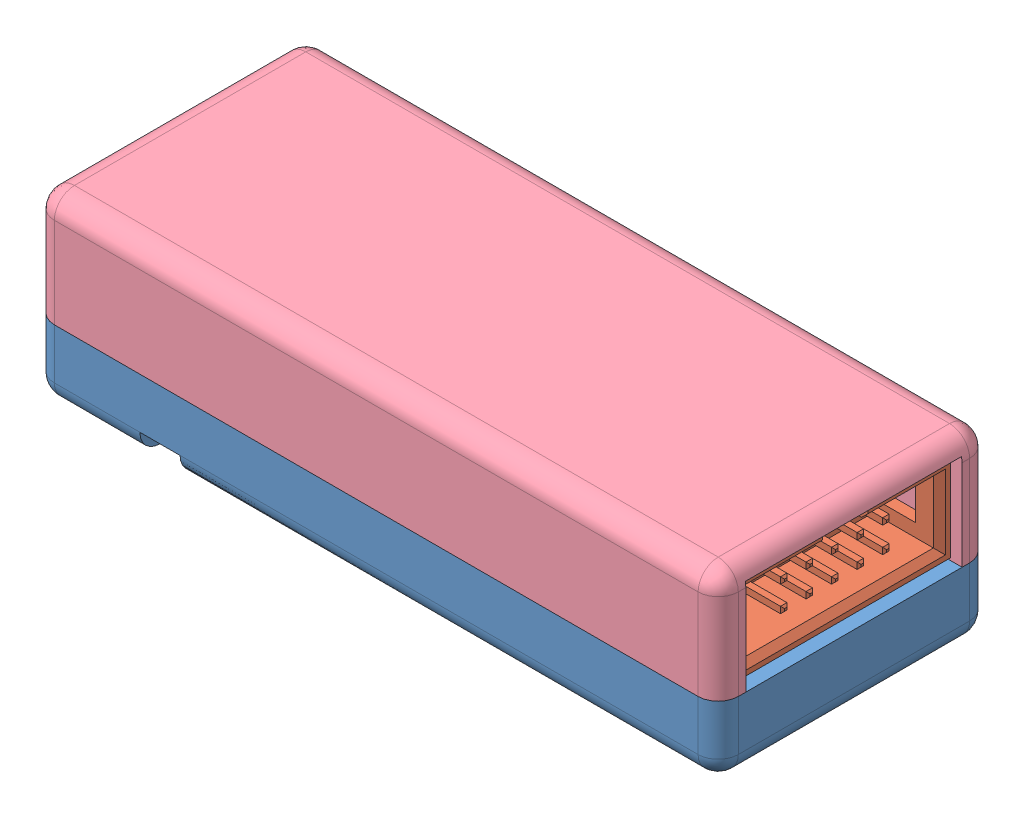
SolidWorks assembly Сборка J-Link Isolated, configuration По умолчанию. Lengths in mm.
Overall size (68 18.11 27).
6 component instances, 5 part files, 7 mates.
Components (placement in the parent):
- Bottom-1: Bottom [По умолчанию] at origin size (68 7 27)
- Board-1: Board [По умолчанию] at (-31.5 6.9786 0) x (0 0 1) z (0 1 0) size (22 66.22 13.13)
- M2X10MM_HEXAGON-1: M2X10MM_HEXAGON [M2X10mm] at (-21.5 0 9) x (0 0 -1) z (0 -1 0) size (3.8 3.8 12.11)
- M2X10MM_HEXAGON-2: M2X10MM_HEXAGON [M2X10mm] at (-21.5 0 -9) x (0 0 -1) z (0 -1 0) size (3.8 3.8 12.11)
- Деталь4^Сборка J-Link Isolated-1: Деталь4^Сборка J-Link Isolated [По умолчанию] at origin (virtual)
- Top-1: Top [По умолчанию] at (0 7 0) size (68 11 27)
Mates (geometry in assembly coordinates):
- Совпадение1: coincident anti-aligned: plane of Bottom-1 through (0 5.4 0) normal (0 1 0); plane of Board-1 through (-30.5 5.4 -11) normal (0 -1 0)
- Концентричный2: concentric aligned: cylinder of Bottom-1 through (23 8.6919 -11) axis (0 -1 0) radius 0.7; cylinder of Board-1 through (23 5.4 -11) axis (0 -1 0) radius 0.75
- Концентричный4: concentric anti-aligned: cylinder of Bottom-1 through (-21.5 0 9) axis (0 1 0) radius 1.2; cylinder of M2X10MM_HEXAGON-1 through (-21.5 0 9) axis (0 -1 0) radius 1
- Совпадение3: coincident anti-aligned: plane of Bottom-1 through (-21.5 2 9) normal (0 -1 0); plane of M2X10MM_HEXAGON-1 through (-19.76 2 9) normal (0 1 0)
- Концентричный5: concentric anti-aligned: cylinder of Bottom-1 through (-21.5 0 -9) axis (0 1 0) radius 1.2; cylinder of M2X10MM_HEXAGON-2 through (-21.5 0 -9) axis (0 -1 0) radius 1
- Совпадение4: coincident anti-aligned: plane of Bottom-1 through (-21.5 2 -9) normal (0 -1 0); plane of M2X10MM_HEXAGON-2 through (-19.76 2 -9) normal (0 1 0)
- Совпадение5: coincident anti-aligned: plane of Bottom-1 through (0 7 0) normal (0 1 0); plane of Top-1 through (0 7 0) normal (0 -1 0)
